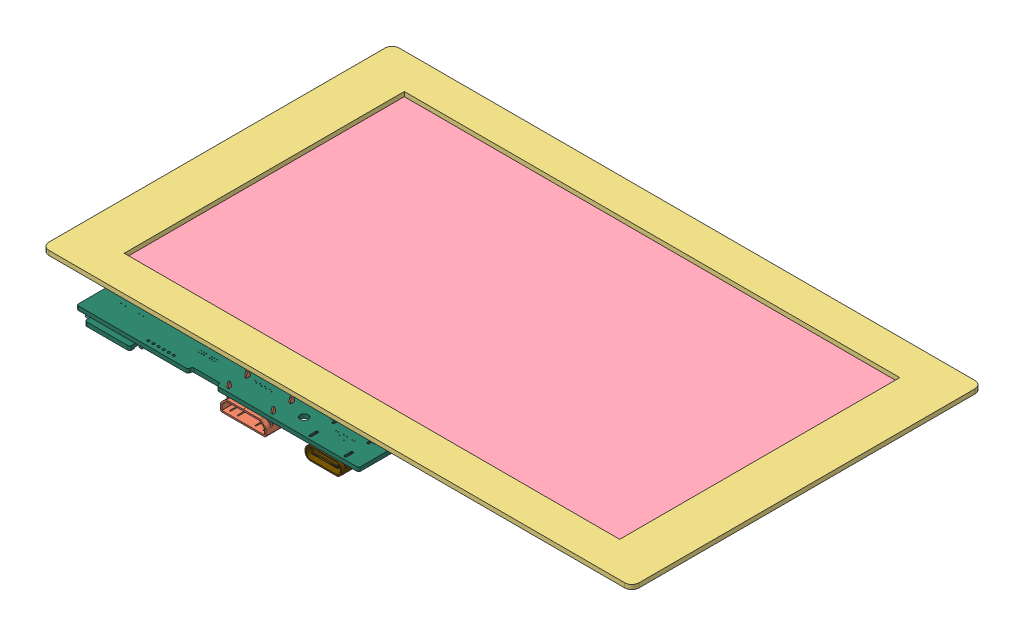
SolidWorks assembly Assembly Center Components, configuration Default. Lengths in mm. (continued)
Components (placement in the parent): (continued)
- Radxa CM3-1: Radxa CM3 [Default] at (-34.1679 -8.7691 -17.6603) x (0 0 -1) z (0 -1 0) size (40.05 55.02 3.7) (continued)
  - EMP_Models-1: EMP_Models [Default] at origin size (39.5 54.73 3.7) (continued)
    - C10-202: C10 [Default] at (-4.7475 1.3019 -1.2) x (-0.707107 -0.707107 0) z (0 0 -1) size (1.1 0.6 0.35)
    - C10-203: C10 [Default] at (0.9 2.95 -1.2) x (0.707107 -0.707107 0) z (0 0 -1) size (1.1 0.6 0.35)
    - C10-204: C10 [Default] at (4.05 11.1 -1.2) x (0 -1 0) z (0 0 -1) size (1.1 0.6 0.35)
    - D1-1: D1 [Default] at (13.3703 9.2021 0) x (-1 0 0) z (0 0 1) size (3.3 1.4 0.8)
    - D1-2: D1 [Default] at (15.4253 4.4887 0) x (0 -1 0) z (0 0 1) size (3.3 1.4 0.8)
    - ED8144-1: ED8144 [Default] at (-15.7 3.95 0) x (0 1 0) z (0 0 1) size (1.77 0.93 0.8)
    - ED8144-2: ED8144 [Default] at (-14.65 -20.2 0) size (1.77 0.93 0.8)
    - ED8144-3: ED8144 [Default] at (-2.4887 24.0177 0) x (0 1 0) z (0 0 1) size (1.77 0.93 0.8)
    - ED8147-1: ED8147 [Default] at (18.2193 9.1971 0) size (2.41 1.24 0.8)
    - ED8144-4: ED8144 [Default] at (17.6586 1.0982 0) x (0 -1 0) z (0 0 1) size (1.77 0.93 0.8)
    - ED8144-5: ED8144 [Default] at (17.6586 2.8762 0) x (0 1 0) z (0 0 1) size (1.77 0.93 0.8)
    - FB1-1: FB1 [Default] at (1.65 9.65 -1.2) x (1 0 0) z (0 0 -1) size (1.7 0.8 0.5)
    - FB1-2: FB1 [Default] at (9.4715 23.3369 0) x (0 1 0) z (0 0 1) size (1.7 0.8 0.5)
    - FB1-3: FB1 [Default] at (10.7443 20.4739 -1.2) x (1 0 0) z (0 0 -1) size (1.7 0.8 0.5)
    - FB1-4: FB1 [Default] at (9.7417 13.5389 -1.2) x (1 0 0) z (0 0 -1) size (1.7 0.8 0.5)
    - FB1-5: FB1 [Default] at (12.05 13.95 -1.2) x (0 -1 0) z (0 0 -1) size (1.7 0.8 0.5)
    - FB1-6: FB1 [Default] at (3.5025 2.1519 -1.2) x (-0.707107 0.707107 0) z (0 0 -1) size (1.7 0.8 0.5)
    - FB5-1: FB5 [Default] at (17.7525 -10.7981 0) x (0 -1 0) z (0 0 1) size (2.08 1.34 0.7)
    - FB5-2: FB5 [Default] at (16.3025 -10.7981 0) x (0 -1 0) z (0 0 1) size (2.08 1.34 0.7)
    - FB5-3: FB5 [Default] at (14.8525 -10.7981 0) x (0 -1 0) z (0 0 1) size (2.08 1.34 0.7)
    - FB5-4: FB5 [Default] at (13.4025 -10.7981 0) x (0 -1 0) z (0 0 1) size (2.08 1.34 0.7)
    - FB9-1: FB9 [Default] at (11.1972 22.9552 0) size (2.8 1.3 0.6)
    - J1-1: J1 [Default] at (11.3212 22.5507 -1.2) x (0 1 0) z (0 0 -1) size (2.84 22.55 1)
    - J90033-1: J90033 [Default] at (-13.7 5.05 0) x (0 1 0) z (0 0 1) size (4.08 2.13 0.5)
    - J90033-2: J90033 [Default] at (-16.8 -18.5 0) x (-1 0 0) z (0 0 1) size (4.08 2.13 0.5)
    - L1-1: L1 [Default] at (9.3525 -25.5481 0) x (0 1 0) z (0 0 1) size (2.78 2.28 1)
    - L10-1: L10 [Default] at (5.8 11.7 0) x (0 1 0) z (0 0 1) size (2.78 2.28 1)
    - L10-2: L10 [Default] at (12.0115 18.7649 0) size (2.78 2.28 1)
    - L10-3: L10 [Default] at (-0.9 20.75 0) x (0 1 0) z (0 0 1) size (2.78 2.28 1)
    - L13-1: L13 [Default] at (-13.7665 -4.2312 0) x (-0.707107 -0.707107 0) z (0 0 1) size (2.83 2.1 1.2)
    - L2-1: L2 [Default] at (-11.1177 21.5067 0) x (-0.707107 -0.707107 0) z (0 0 1) size (1.1 0.6 0.35)
    - L2-2: L2 [Default] at (-11.7527 23.4117 0) x (-1 0 0) z (0 0 1) size (1.1 0.6 0.35)
    - L10-4: L10 [Default] at (-17.3475 4.7519 0) x (0 -1 0) z (0 0 1) size (2.78 2.28 1)
    - L10-5: L10 [Default] at (18.3025 -19.6481 0) x (-1 0 0) z (0 0 1) size (2.78 2.28 1)
    - L10-6: L10 [Default] at (9.2 12.15 0) x (-1 0 0) z (0 0 1) size (2.78 2.28 1)
    - L10-7: L10 [Default] at (-0.85 16.7 0) x (0 1 0) z (0 0 1) size (2.78 2.28 1)
    - LED1-1: LED1 [Default] at (-2.8224 26.4941 0) x (-1 0 0) z (0 0 1) size (2.95 1.43 0.6)
    - M1-1: M1 [Default] at (-12.0975 -25.5981 -1.2) x (-1 0 0) z (0 0 -1) size (3.45 3.45 0.1)
    - M1-2: M1 [Default] at (12.2025 25.6519 0) size (3.45 3.45 0.1)
    - M1-3: M1 [Default] at (-12.0975 -25.5981 0) size (3.45 3.45 0.1)
    - M1-4: M1 [Default] at (12.2025 25.6519 -1.2) x (-1 0 0) z (0 0 -1) size (3.45 3.45 0.1)
    - Q4-1: Q4 [Default] at (-8.45 5.5 -1.2) x (-1 0 0) z (0 0 -1) size (1.27 1.32 0.8)
    - Q5-1: Q5 [Default] at (-7.3 23.05 0) size (3.35 3.3 1)
    - Q5-2: Q5 [Default] at (17 -3.9 0) x (-1 0 0) z (0 0 1) size (3.35 3.3 1)
    - R1-1: R1 [Default] at (6.8025 -4.5481 -1.2) x (1 0 0) z (0 0 -1) size (1.7 0.9 0.5)
    - L2-3: L2 [Default] at (12.9303 4.6718 -1.2) x (0 -1 0) z (0 0 -1) size (1.1 0.6 0.35)
    - L2-4: L2 [Default] at (17.75 -11.3 -1.2) x (0 1 0) z (0 0 -1) size (1.1 0.6 0.35)
    - L2-5: L2 [Default] at (17.75 -12.45 -1.2) x (0 1 0) z (0 0 -1) size (1.1 0.6 0.35)
    - L2-6: L2 [Default] at (15.7025 -17.9981 -1.2) x (0 1 0) z (0 0 -1) size (1.1 0.6 0.35)
    - L2-7: L2 [Default] at (18.45 -11.3 -1.2) x (0 1 0) z (0 0 -1) size (1.1 0.6 0.35)
    - L2-8: L2 [Default] at (18.45 -12.45 -1.2) x (0 1 0) z (0 0 -1) size (1.1 0.6 0.35)
    - L2-9: L2 [Default] at (15.0525 -17.9981 -1.2) x (0 1 0) z (0 0 -1) size (1.1 0.6 0.35)
    - L2-10: L2 [Default] at (15.0525 -19.1481 -1.2) x (0 1 0) z (0 0 -1) size (1.1 0.6 0.35)
    - L2-11: L2 [Default] at (13.7525 -17.9981 -1.2) x (0 1 0) z (0 0 -1) size (1.1 0.6 0.35)
    - L2-12: L2 [Default] at (13.7525 -19.1481 -1.2) x (0 1 0) z (0 0 -1) size (1.1 0.6 0.35)
    - R1-2: R1 [Default] at (12.7025 -9.6481 0) size (1.7 0.9 0.5)
    - L2-13: L2 [Default] at (0.4486 12.9437 -1.2) x (0 1 0) z (0 0 -1) size (1.1 0.6 0.35)
    - R1-3: R1 [Default] at (13.1025 -8.2481 0) x (0 -1 0) z (0 0 1) size (1.7 0.9 0.5)
    - L2-14: L2 [Default] at (14.4025 -17.9981 -1.2) x (0 1 0) z (0 0 -1) size (1.1 0.6 0.35)
    - L2-15: L2 [Default] at (14.4025 -19.1481 -1.2) x (0 1 0) z (0 0 -1) size (1.1 0.6 0.35)
    - R1-4: R1 [Default] at (12.9525 -11.8481 -1.2) x (-1 0 0) z (0 0 -1) size (1.7 0.9 0.5)
    - R1-5: R1 [Default] at (18.8525 -19.1481 -1.2) x (-1 0 0) z (0 0 -1) size (1.7 0.9 0.5)
    - L2-16: L2 [Default] at (11.8525 -13.8481 -1.2) x (0 -1 0) z (0 0 -1) size (1.1 0.6 0.35)
    - L2-17: L2 [Default] at (11.6025 -15.0981 -1.2) x (1 0 0) z (0 0 -1) size (1.1 0.6 0.35)
    - L2-18: L2 [Default] at (11.2025 -13.8481 -1.2) x (0 -1 0) z (0 0 -1) size (1.1 0.6 0.35)
    - L2-19: L2 [Default] at (11.7525 -16.2481 -1.2) x (-1 0 0) z (0 0 -1) size (1.1 0.6 0.35)
    - L2-20: L2 [Default] at (13.9025 -20.1981 0) x (0 -1 0) z (0 0 1) size (1.1 0.6 0.35)
    - R1-6: R1 [Default] at (11.8808 6.1274 0) size (1.7 0.9 0.5)
    - R1-7: R1 [Default] at (10.5014 7.0239 0) x (0 1 0) z (0 0 1) size (1.7 0.9 0.5)
    - L2-21: L2 [Default] at (-10.0048 -2.9217 0) x (-1 0 0) z (0 0 1) size (1.1 0.6 0.35)
    - L2-22: L2 [Default] at (-11.25 4.25 0) x (-0.707107 0.707107 0) z (0 0 1) size (1.1 0.6 0.35)
    - L2-23: L2 [Default] at (-7.55 2.1989 -1.2) x (1 0 0) z (0 0 -1) size (1.1 0.6 0.35)
    - L2-24: L2 [Default] at (18.2 -17.4 -1.2) x (-1 0 0) z (0 0 -1) size (1.1 0.6 0.35)
    - L2-25: L2 [Default] at (18.2 -16.75 -1.2) x (-1 0 0) z (0 0 -1) size (1.1 0.6 0.35)
    - L2-26: L2 [Default] at (19.25 -17.15 -1.2) x (0 -1 0) z (0 0 -1) size (1.1 0.6 0.35)
    - L2-27: L2 [Default] at (-13.3547 0.5177 0) x (-0.707107 -0.707107 0) z (0 0 1) size (1.1 0.6 0.35)
    - L2-28: L2 [Default] at (-3.95 9.75 0) x (0.707107 0.707107 0) z (0 0 1) size (1.1 0.6 0.35)
    - L2-29: L2 [Default] at (-7.45 4.9 -1.2) x (0 1 0) z (0 0 -1) size (1.1 0.6 0.35)
    - L2-30: L2 [Default] at (-3.35 10.8 0) x (0 1 0) z (0 0 1) size (1.1 0.6 0.35)
    - L2-31: L2 [Default] at (-8.9 -1.05 -1.2) x (0 1 0) z (0 0 -1) size (1.1 0.6 0.35)
    - L2-32: L2 [Default] at (-9.7407 -0.3884 -1.2) x (-1 0 0) z (0 0 -1) size (1.1 0.6 0.35)
    - L2-33: L2 [Default] at (1.5025 -5.4481 -1.2) x (-0.707107 -0.707107 0) z (0 0 -1) size (1.1 0.6 0.35)
    - L2-34: L2 [Default] at (-9.7625 1.3757 -1.2) x (1 0 0) z (0 0 -1) size (1.1 0.6 0.35)
    - L2-35: L2 [Default] at (-9.7722 0.251 -1.2) x (1 0 0) z (0 0 -1) size (1.1 0.6 0.35)
    - L2-36: L2 [Default] at (8.8525 -3.8481 -1.2) x (1 0 0) z (0 0 -1) size (1.1 0.6 0.35)
    - L2-37: L2 [Default] at (8.8525 -4.4981 -1.2) x (1 0 0) z (0 0 -1) size (1.1 0.6 0.35)
    - R24-1: R24 [Default] at (13.5019 5.7507 0) x (0 -1 0) z (0 0 1) size (2.5 1.3 0.6)
    - L2-38: L2 [Default] at (8.8525 -5.1481 -1.2) x (1 0 0) z (0 0 -1) size (1.1 0.6 0.35)
    - R1-8: R1 [Default] at (11.8808 7.9054 0) x (-1 0 0) z (0 0 1) size (1.7 0.9 0.5)
    - L2-39: L2 [Default] at (8.839 -5.6572 -1.2) x (-1 0 0) z (0 0 -1) size (1.1 0.6 0.35)
    - L2-40: L2 [Default] at (13.5019 8.1637 0) size (1.1 0.6 0.35)
    - R1-9: R1 [Default] at (11.8808 7.0164 0) x (-1 0 0) z (0 0 1) size (1.7 0.9 0.5)
    - L2-41: L2 [Default] at (1.9025 -4.5981 -1.2) x (-0.707107 0.707107 0) z (0 0 -1) size (1.1 0.6 0.35)
    - R1-10: R1 [Default] at (12.4 10.2 -1.2) x (-1 0 0) z (0 0 -1) size (1.7 0.9 0.5)
    - R1-11: R1 [Default] at (12.4278 9.235 -1.2) x (-1 0 0) z (0 0 -1) size (1.7 0.9 0.5)
    - L2-42: L2 [Default] at (0.0025 12.7519 0) x (0.707107 0.707107 0) z (0 0 1) size (1.1 0.6 0.35)
    - L2-43: L2 [Default] at (0.4393 12.3013 0) x (0.707107 0.707107 0) z (0 0 1) size (1.1 0.6 0.35)
    - L2-44: L2 [Default] at (0.9525 11.8019 0) x (0.707107 0.707107 0) z (0 0 1) size (1.1 0.6 0.35)
    - L2-45: L2 [Default] at (1.3881 11.3747 0) x (0.707107 0.707107 0) z (0 0 1) size (1.1 0.6 0.35)
    - L2-46: L2 [Default] at (1.9025 10.8519 0) x (0.707107 0.707107 0) z (0 0 1) size (1.1 0.6 0.35)
    - L2-47: L2 [Default] at (2.3296 10.4351 0) x (0.707107 0.707107 0) z (0 0 1) size (1.1 0.6 0.35)
    - L2-48: L2 [Default] at (2.8525 9.9019 0) x (0.707107 0.707107 0) z (0 0 1) size (1.1 0.6 0.35)
    - L2-49: L2 [Default] at (3.2748 9.4731 0) x (0.707107 0.707107 0) z (0 0 1) size (1.1 0.6 0.35)
    - L2-50: L2 [Default] at (-4.75 10.35 0) x (-1 0 0) z (0 0 1) size (1.1 0.6 0.35)
    - L2-51: L2 [Default] at (1.1909 6.5961 -1.2) x (0 -1 0) z (0 0 -1) size (1.1 0.6 0.35)
    - L2-52: L2 [Default] at (10.3525 2.1019 0) x (-0.707107 0.707107 0) z (0 0 1) size (1.1 0.6 0.35)
    - R1-12: R1 [Default] at (9.9432 9.4653 0) size (1.7 0.9 0.5)
    - R1-13: R1 [Default] at (9.5622 8.0683 0) x (0 -1 0) z (0 0 1) size (1.7 0.9 0.5)
    - L2-53: L2 [Default] at (-8.7065 -3.7391 0) size (1.1 0.6 0.35)
    - L2-54: L2 [Default] at (-8.7065 -4.3741 0) size (1.1 0.6 0.35)
    - L2-55: L2 [Default] at (-6.5975 -2.9981 -1.2) x (-0.707107 -0.707107 0) z (0 0 -1) size (1.1 0.6 0.35)
    - R1-14: R1 [Default] at (-15.4372 0.8153 0) x (-1 0 0) z (0 0 1) size (1.7 0.9 0.5)
    - L2-56: L2 [Default] at (-18.76 -2.973 0) x (-0.707107 0.707107 0) z (0 0 1) size (1.1 0.6 0.35)
    - R1-15: R1 [Default] at (-15.0359 2.0509 0) x (0 1 0) z (0 0 1) size (1.7 0.9 0.5)
    - L2-57: L2 [Default] at (-5.15 9.75 0) x (-1 0 0) z (0 0 1) size (1.1 0.6 0.35)
    - L2-58: L2 [Default] at (-18.3381 -2.5736 0) x (0.707107 -0.707107 0) z (0 0 1) size (1.1 0.6 0.35)
    - L2-59: L2 [Default] at (5.8025 -20.8481 -1.2) x (1 0 0) z (0 0 -1) size (1.1 0.6 0.35)
    - L2-60: L2 [Default] at (5.8025 -20.1981 -1.2) x (1 0 0) z (0 0 -1) size (1.1 0.6 0.35)
    - R24-2: R24 [Default] at (11.9025 -23.7981 -1.2) x (-1 0 0) z (0 0 -1) size (2.5 1.3 0.6)
    - R1-16: R1 [Default] at (-13.55 -21.25 -1.2) x (1 0 0) z (0 0 -1) size (1.7 0.9 0.5)
    - R24-3: R24 [Default] at (7.0025 -26.5481 -1.2) x (-1 0 0) z (0 0 -1) size (2.5 1.3 0.6)
    - R1-17: R1 [Default] at (-13.55 -20.3 -1.2) x (1 0 0) z (0 0 -1) size (1.7 0.9 0.5)
    - L2-61: L2 [Default] at (11.5525 -21.7481 0) size (1.1 0.6 0.35)
    - L2-62: L2 [Default] at (12.7525 -26.2481 -1.2) x (1 0 0) z (0 0 -1) size (1.1 0.6 0.35)
    - L2-63: L2 [Default] at (-18.4 -16.6 -1.2) x (1 0 0) z (0 0 -1) size (1.1 0.6 0.35)
    - L2-64: L2 [Default] at (-1.6 13.75 0) x (0 1 0) z (0 0 1) size (1.1 0.6 0.35)
    - L2-65: L2 [Default] at (13.9525 -26.8981 0) size (1.1 0.6 0.35)
    - L2-66: L2 [Default] at (-12.014 6.1193 -1.2) x (0 1 0) z (0 0 -1) size (1.1 0.6 0.35)
    - L2-67: L2 [Default] at (-10.4 5.9 -1.2) x (0 1 0) z (0 0 -1) size (1.1 0.6 0.35)
    - L2-68: L2 [Default] at (-12.6417 6.1168 -1.2) x (0 1 0) z (0 0 -1) size (1.1 0.6 0.35)
    - L2-69: L2 [Default] at (-11.4087 6.1174 -1.2) x (0 1 0) z (0 0 -1) size (1.1 0.6 0.35)
    - L2-70: L2 [Default] at (-12.6469 -1.643 -1.2) x (1 0 0) z (0 0 -1) size (1.1 0.6 0.35)
    - L2-71: L2 [Default] at (13.1198 7.7736 -1.2) x (1 0 0) z (0 0 -1) size (1.1 0.6 0.35)
    - L2-72: L2 [Default] at (-16.9 -11.65 -1.2) x (-1 0 0) z (0 0 -1) size (1.1 0.6 0.35)
    - L2-73: L2 [Default] at (-18.1 -11.65 -1.2) x (1 0 0) z (0 0 -1) size (1.1 0.6 0.35)
    - L2-74: L2 [Default] at (-15.6 -15.95 -1.2) x (-1 0 0) z (0 0 -1) size (1.1 0.6 0.35)
    - L2-75: L2 [Default] at (-12.55 0.45 -1.2) x (-1 0 0) z (0 0 -1) size (1.1 0.6 0.35)
    - L2-76: L2 [Default] at (-13.55 0.45 -1.2) x (-1 0 0) z (0 0 -1) size (1.1 0.6 0.35)
    - R24-4: R24 [Default] at (-14.4732 17.1388 -1.2) x (0 1 0) z (0 0 -1) size (2.5 1.3 0.6)
    - L2-77: L2 [Default] at (-17.707 19.6733 -1.2) x (1 0 0) z (0 0 -1) size (1.1 0.6 0.35)
    - L2-78: L2 [Default] at (13.1107 8.3605 -1.2) x (1 0 0) z (0 0 -1) size (1.1 0.6 0.35)
    - L2-79: L2 [Default] at (-17.7116 19.1714 -1.2) x (-1 0 0) z (0 0 -1) size (1.1 0.6 0.35)
    - L2-80: L2 [Default] at (-12.999 2.1325 0) x (-1 0 0) z (0 0 1) size (1.1 0.6 0.35)
    - L2-81: L2 [Default] at (-5.9125 16.7079 0) x (0 1 0) z (0 0 1) size (1.1 0.6 0.35)
    - L2-82: L2 [Default] at (-18.8975 5.2019 0) x (0 -1 0) z (0 0 1) size (1.1 0.6 0.35)
    - R1-18: R1 [Default] at (-17.0263 0.7967 0) size (1.7 0.9 0.5)
    - R1-19: R1 [Default] at (-16.2916 2.0337 0) x (0 1 0) z (0 0 1) size (1.7 0.9 0.5)
    - L2-83: L2 [Default] at (-11.7975 6.8019 0) size (1.1 0.6 0.35)
    - L2-84: L2 [Default] at (18.85 -12.45 0) size (1.1 0.6 0.35)
    - L2-85: L2 [Default] at (18.85 -11.8 0) size (1.1 0.6 0.35)
    - L2-86: L2 [Default] at (12.2953 4.6718 -1.2) x (0 -1 0) z (0 0 -1) size (1.1 0.6 0.35)
    - L2-87: L2 [Default] at (18.85 -13.1 0) size (1.1 0.6 0.35)
    - L2-88: L2 [Default] at (18.1 -0.6 0) x (0 1 0) z (0 0 1) size (1.1 0.6 0.35)
    - L2-89: L2 [Default] at (17.45 -0.6 0) x (0 1 0) z (0 0 1) size (1.1 0.6 0.35)
    - L2-90: L2 [Default] at (18.2 -15.45 -1.2) x (1 0 0) z (0 0 -1) size (1.1 0.6 0.35)
    - L2-91: L2 [Default] at (9.0525 1.2019 -1.2) x (-1 0 0) z (0 0 -1) size (1.1 0.6 0.35)
    - L2-92: L2 [Default] at (-10.2001 3.3697 -1.2) x (0 1 0) z (0 0 -1) size (1.1 0.6 0.35)
    - L2-93: L2 [Default] at (-16.15 -20.2 0) size (1.1 0.6 0.35)
    - R24-5: R24 [Default] at (-8.1 25.45 0) x (-1 0 0) z (0 0 1) size (2.5 1.3 0.6)
    - L2-94: L2 [Default] at (11.7 13.4 0) x (0 1 0) z (0 0 1) size (1.1 0.6 0.35)
    - L2-95: L2 [Default] at (3.95 11.85 0) x (-1 0 0) z (0 0 1) size (1.1 0.6 0.35)
    - L2-96: L2 [Default] at (10.8685 18.0306 -1.2) x (-1 0 0) z (0 0 -1) size (1.1 0.6 0.35)
    - L2-97: L2 [Default] at (8.5825 18.5109 -1.2) x (-1 0 0) z (0 0 -1) size (1.1 0.6 0.35)
    - L2-98: L2 [Default] at (5.9323 23.8177 0) x (0 -1 0) z (0 0 1) size (1.1 0.6 0.35)
    - L2-99: L2 [Default] at (5.2823 23.8177 0) x (0 -1 0) z (0 0 1) size (1.1 0.6 0.35)
    - L2-100: L2 [Default] at (-8.8 24.55 0) x (-1 0 0) z (0 0 1) size (1.1 0.6 0.35)
    - R9216-1: R9216 [Default] at (3.3 18.2 -1.2) x (1 0 0) z (0 0 -1) size (3.6 2.1 0.8)
    - L2-101: L2 [Default] at (-0.3818 13.9135 -1.2) x (0 1 0) z (0 0 -1) size (1.1 0.6 0.35)
    - L2-102: L2 [Default] at (0.45 16.7 -1.2) x (-1 0 0) z (0 0 -1) size (1.1 0.6 0.35)
    - L2-103: L2 [Default] at (-0.3818 14.9291 -1.2) x (0 1 0) z (0 0 -1) size (1.1 0.6 0.35)
    - L2-104: L2 [Default] at (0.55 14.45 -1.2) x (-1 0 0) z (0 0 -1) size (1.1 0.6 0.35)
    - L2-105: L2 [Default] at (-1.1 14.15 0) x (0 -1 0) z (0 0 1) size (1.1 0.6 0.35)
    - L2-106: L2 [Default] at (0.75 14.6 0) x (0 1 0) z (0 0 1) size (1.1 0.6 0.35)
    - L2-107: L2 [Default] at (-3.9887 23.8177 0) x (0 1 0) z (0 0 1) size (1.1 0.6 0.35)
    - R9216-2: R9216 [Default] at (16.5683 7.4937 0) x (-1 0 0) z (0 0 1) size (3.6 2.1 0.8)
    - L2-108: L2 [Default] at (-18.0618 -3.6891 0) x (0.707107 -0.707107 0) z (0 0 1) size (1.1 0.6 0.35)
    - L2-109: L2 [Default] at (-16.8694 -1.2155 0) x (-0.707107 -0.707107 0) z (0 0 1) size (1.1 0.6 0.35)
    - L2-110: L2 [Default] at (-18.4855 -4.1201 0) x (0.707107 -0.707107 0) z (0 0 1) size (1.1 0.6 0.35)
    - R1-20: R1 [Default] at (4.2 12.6 -1.2) x (0 1 0) z (0 0 -1) size (1.7 0.9 0.5)
    - R1-21: R1 [Default] at (2.6 12.6 -1.2) x (0 1 0) z (0 0 -1) size (1.7 0.9 0.5)
    - R1-22: R1 [Default] at (5 12.6 -1.2) x (0 1 0) z (0 0 -1) size (1.7 0.9 0.5)
    - R1-23: R1 [Default] at (9.8 14.3 -1.2) x (-1 0 0) z (0 0 -1) size (1.7 0.9 0.5)
    - R1-24: R1 [Default] at (-18.35 1.2 0) x (0 1 0) z (0 0 1) size (1.7 0.9 0.5)
    - R1-25: R1 [Default] at (3.4 12.6 -1.2) x (0 1 0) z (0 0 -1) size (1.7 0.9 0.5)
    - L2-111: L2 [Default] at (-3.1812 25.4157 0) size (1.1 0.6 0.35)
    - L2-112: L2 [Default] at (15.7205 1.3062 0) size (1.1 0.6 0.35)
    - L2-113: L2 [Default] at (15.7205 1.9412 0) size (1.1 0.6 0.35)
    - L2-114: L2 [Default] at (14.7219 1.3075 0) x (-1 0 0) z (0 0 1) size (1.1 0.6 0.35)
    - L2-115: L2 [Default] at (14.9 -3.05 0) x (0 -1 0) z (0 0 1) size (1.1 0.6 0.35)
    - L2-116: L2 [Default] at (17.7 -1.55 0) size (1.1 0.6 0.35)
    - L2-117: L2 [Default] at (-7.95 26.5 0) x (-1 0 0) z (0 0 1) size (1.1 0.6 0.35)
    - L2-118: L2 [Default] at (-9 1.15 -1.2) x (0 1 0) z (0 0 -1) size (1.1 0.6 0.35)
    - L2-119: L2 [Default] at (17.5 -14.2 -1.2) x (-1 0 0) z (0 0 -1) size (1.1 0.6 0.35)
    - L2-120: L2 [Default] at (13.1025 -19.1481 -1.2) x (0 1 0) z (0 0 -1) size (1.1 0.6 0.35)
    - L2-121: L2 [Default] at (19.15 -11.3 -1.2) x (0 1 0) z (0 0 -1) size (1.1 0.6 0.35)
    - L2-122: L2 [Default] at (19.15 -12.45 -1.2) x (0 1 0) z (0 0 -1) size (1.1 0.6 0.35)
    - L2-123: L2 [Default] at (18.7525 -17.9981 0) size (1.1 0.6 0.35)
    - L2-124: L2 [Default] at (15.2025 -20.1981 0) x (0 -1 0) z (0 0 1) size (1.1 0.6 0.35)
    - L2-125: L2 [Default] at (14.0025 -20.0481 -1.2) x (1 0 0) z (0 0 -1) size (1.1 0.6 0.35)
    - TP1-1: TP1 [Default] at (-12.0342 7.0446 -1.2) x (-1 0 0) z (0 0 -1) size (1 1 0.1)
    - TP1-2: TP1 [Default] at (18.7 0.35 0) size (1 1 0.1)
    - TP1-3: TP1 [Default] at (-7 3 -1.2) x (-0.707107 0.707107 0) z (0 0 -1) size (1 1 0.1)
    - TP1-4: TP1 [Default] at (18.75 13.45 -1.2) x (-1 0 0) z (0 0 -1) size (1 1 0.1)
    - TP1-5: TP1 [Default] at (19.4 9.05 -1.2) x (-1 0 0) z (0 0 -1) size (1 1 0.1)
    - TP1-6: TP1 [Default] at (19.4 10.6 -1.2) x (-1 0 0) z (0 0 -1) size (1 1 0.1)
    - TP1-7: TP1 [Default] at (-18.6 -15.75 -1.2) x (-1 0 0) z (0 0 -1) size (1 1 0.1)
    - TP1-8: TP1 [Default] at (-17.5 -15.75 -1.2) x (-1 0 0) z (0 0 -1) size (1 1 0.1)
    - TP1-9: TP1 [Default] at (14.35 -10.85 -1.2) x (-1 0 0) z (0 0 -1) size (1 1 0.1)
    - TP1-10: TP1 [Default] at (-8.8451 3.2927 -1.2) x (-1 0 0) z (0 0 -1) size (1 1 0.1)
    - TP1-11: TP1 [Default] at (4.5413 20.3907 -1.2) x (-1 0 0) z (0 0 -1) size (1 1 0.1)
    - TP1-12: TP1 [Default] at (18.6825 1.3989 0) size (1 1 0.1)
    - TP1-13: TP1 [Default] at (18.6825 2.4489 0) size (1 1 0.1)
    - U1-1: U1 [Default] at (-0.1975 0.4519 0) x (-0.707107 0.707107 0) z (0 0 1) size (18.71 17.21 1.1)
    - U2-1: U2 [Default] at (-1.0248 -19.8218 0) x (0 -1 0) z (0 0 1) size (13.49 18.53 1)
    - U3-1: U3 [Default] at (12.9025 -23.7481 0) x (0 -1 0) z (0 0 1) size (4.03 3.13 1)
    - U3-2: U3 [Default] at (-18.15 -19.4 -1.2) x (1 0 0) z (0 0 -1) size (4.03 3.13 1)
    - U4300-1: U4300 [Default] at (-16.9 -13.45 0) x (-1 0 0) z (0 0 1) size (5.99 7 1.2)
    - U4301-1: U4301 [Default] at (5.2805 18.1299 0) x (0 1 0) z (0 0 1) size (8.35 8.35 0.8)
    - U4302-1: U4302 [Default] at (-16.4535 -5.0091 0) x (0.707107 0.707107 0) z (0 0 1) size (1.93 2.38 0.8)
    - U5-1: U5 [Default] at (-7.6975 14.2519 -1.2) x (1 0 0) z (0 0 -1) size (11.63 13.5 1.2)
    - U7-1: U7 [Default] at (14.2608 3.741 0) x (0 -1 0) z (0 0 1) size (2.08 2.45 0.7)
    - U8-1: U8 [Default] at (-12.9975 13.9519 0) x (0 -1 0) z (0 0 1) size (13.66 12.7 1.3)
    - U9-1: U9 [Default] at (15.3025 -15.6981 0) x (0 -1 0) z (0 0 1) size (5.84 5.5 1)
    - U3-3: U3 [Default] at (13.5 0.3 0) size (4.03 3.13 1)
    - Y1-1: Y1 [Default] at (-4.2838 13.1005 0) x (-1 0 0) z (0 0 1) size (3.6 3.57 1.2)
    - Y1-2: Y1 [Default] at (-17.6116 16.6641 -1.2) x (-1 0 0) z (0 0 -1) size (3.6 3.57 1.2)
    - Y1-3: Y1 [Default] at (17.8 -7.6 0) x (0 -1 0) z (0 0 1) size (3.6 3.57 1.2)
    - Y4-1: Y4 [Default] at (-0.81 24.6548 0) size (3.6 1.7 1.2)
  - Board_outline(1)-1: Board_outline(1) [Default] at origin size (40.05 55.02 1.2)
- User Library-CR1225 v1-1: User Library-CR1225 v1 [Default] at (-65.8849 -7.0512 19.9145) x (0 0 -1) z (0 -1 0) size (12.4 12.4 2.5)
  - refine_Revolution001-1: refine_Revolution001 [Default] at (0 0 2.5) x (1 0 0) z (0 1 0) size (10.2 0.85 10.2)
  - refine_Cut001-1: refine_Cut001 [Default] at (0 1 2.5) x (1 0 0) z (0 1 0) size (12.4 2.5 12.4)
- 5040500491 v1-1: 5040500491 v1 [Default] at (-31.1609 -7.15 36.6709) x (-1 0 0) z (0 -1 0) size (10.55 6.44 2)
  - 5040500491-1: 5040500491 [Default] at origin size (10.55 6.44 2)
- DF40C-100DS-1: DF40C-100DS [Default] at (-37.655 -6.2 -0.495) x (0 0 -1) z (-1 0 0) size (3.49 2 22.61)
- DF40C-100DS-2: DF40C-100DS [Default] at (-37.655 -6.2 -34.495) x (0 0 -1) z (-1 0 0) size (3.49 2 22.61)
- Micro SD-Card-1: Micro SD-Card [Default] at (-52.45 -7.1 39.52) x (0 0 -1) z (-1 0 0) size (15 1.01 11)
- CUI_DEVICES_SJ-43516-SMT-TR-1: CUI_DEVICES_SJ-43516-SMT-TR [Default] at (-2.55 -8.65 -45.17) x (0 0 -1) z (-1 0 0) size (19.2 5.8 9)
- PCIe Slot  v1-1: PCIe Slot  v1 [Default] at (-9.09 -6.1502 6.7) x (-1 0 0) z (0 0 1) size (22 4.8 8.55)
- 1054500101 v1-1: 1054500101 v1 [Default] at (0 -7.7798 41.669) x (1 0 0) z (0 -1 0) size (8.94 7.9 3.96)
- 502570-0893 v1-1: 502570-0893 v1 [Default] at (-97.1844 -7.0502 -24.8743) x (1 0 0) z (0 -1 0) size (13.8 15.5 1.8)
- 9774025243R (rev1) v1-1: 9774025243R (rev1) v1 [Default] at (0 -52.8238 2.1762) x (1 0 0) z (0 -1 0) size (4.35 4.35 3.9)
- DF40C-100DS-3: DF40C-100DS [Default] at (-9.8603 -6.2 -23.511) x (1 0 0) z (0 0 -1) size (3.49 2 22.61)
- 5051100892 v1-1: 5051100892 v1 [Default] at (-65.4404 -6.1942 -19.6945) x (0 0 1) z (1 0 0) size (9.5 1.9 5.3)
- keystone-PN1072TR v1-1: keystone-PN1072TR v1 [Default] at (-72.6801 -0.2846 31.6836) x (1 0 0) z (0 0 -1) size (10.39 4.4 15.9)
- TPS65987DDHRSHR--3DModel-STEP-56544 v1-1: TPS65987DDHRSHR--3DModel-STEP-56544 v1 [Default] at (-12.5607 -6.1 22.9561) x (-1 0 0) z (0 0 1) size (7 1 7)
- TPD4E05U06DQAR--3DModel-STEP-56544 v1-1: TPD4E05U06DQAR--3DModel-STEP-56544 v1 [Default] at (4.7671 -6.1 32.9073) x (0 0 1) z (1 0 0) size (1 0.55 2.5)
- TPD4E05U06DQAR--3DModel-STEP-56544 v1-2: TPD4E05U06DQAR--3DModel-STEP-56544 v1 [Default] at (-3.01 -6.1 32.9073) x (0 0 1) z (1 0 0) size (1 0.55 2.5)
- TSIC 306 SOP-8--3DModel-STEP-510211 v1-1: TSIC 306 SOP-8--3DModel-STEP-510211 v1 [Default] at (-60.1923 -6.1499 6.8931) x (-1 0 0) z (0 0 1) size (5.99 1.73 4.93)
- 5034801700 v1-1: 5034801700 v1 [Default] at (6.9127 -6.1711 10.2732) x (0 0 1) z (1 0 0) size (10.2 1.87 3.6)
- 5034801700 v1-2: 5034801700 v1 [Default] at (-25.1264 -6.1711 10.2943) x (0 0 -1) z (-1 0 0) size (10.2 1.87 3.6)
- VLCF4020T-220MR56--3DModel-STEP-56544 v1-1: VLCF4020T-220MR56--3DModel-STEP-56544 v1 [Default] at (-60.5998 -6.1052 -39.9462) x (0 0 -1) z (-1 0 0) size (4 2.02 4.05)
- Heatsink-V2 v1-1: Heatsink-V2 v1 [Default] at (-21.2372 -13.3527 3.8484) x (0 0 -1) z (1 0 0) size (46.85 6 53)
- QFN_GEFLRV_CIR v1-1: QFN_GEFLRV_CIR v1 [Default] at (0.5729 -5.758 -18.9632) x (1 0 0) z (0 -1 0) size (5 5 0.99)
- 505110-3091 v1-1: 505110-3091 v1 [Default] at (-70.5178 -6.0871 -0.2937) x (0 0 1) z (1 0 0) size (20.5 1.9 5.3)
- ASPI-0630HI v1-1: ASPI-0630HI v1 [Default] at (-31.1721 -7.6525 20.8058) x (-1 0 0) z (0 0 1) size (7.2 3 6.65)
- Retro Lite CM5 (Latest)-18-1: Retro Lite CM5 (Latest)-18 [Default] at origin size (60.98 9.58 0.4)
- Retro Lite CM5 Carrier Board_CM5IO_Mapping_X2.0 v3-1: Retro Lite CM5 Carrier Board_CM5IO_Mapping_X2.0 v3 [Default] at (-1.05 -5.1782 42.5) x (-1 0 0) z (0 -1 0) size (82.67 91.25 0.97)
  - Retro Lite CM5 Carrier Board_CM5IO_Mapping_X2.0 v3(2)^Retro Lite CM5 Carrier Board_CM5IO_Mapping_X2.0 v3-1: Retro Lite CM5 Carrier Board_CM5IO_Mapping_X2.0 v3(2)^Retro Lite CM5 Carrier Board_CM5IO_Mapping_X2.0 v3 [Default] at origin size (82.67 91.25 0.97) (virtual)
    - Board^Retro Lite CM5 Carrier Board_CM5IO_Mapping_X2.0 v3(2)_Retro Lite CM5 Carrier Board_CM5IO_Mapping_X2.0 v3-1: Board^Retro Lite CM5 Carrier Board_CM5IO_Mapping_X2.0 v3(2)_Retro Lite CM5 Carrier Board_CM5IO_Mapping_X2.0 v3 [Default] at origin size (82.67 91.25 0.97) (virtual)
Mates (geometry in assembly coordinates):
- Concentric1: concentric aligned: cylinder of Retro Lite CM5 Carrier Board_CM5IO_Mapping_X2.0 v2 (1)-1/Board (36)-1 through (-72.8 -5.1782 18.5) axis (0 -1 0) radius 1; cylinder of Retro Lite CM5 Carrier Board_CM5IO_Mapping_X2.0 v3-1/Retro Lite CM5 Carrier Board_CM5IO_Mapping_X2.0 v3(2)^Retro Lite CM5 Carrier Board_CM5IO_Mapping_X2.0 v3-1/Board^Retro Lite CM5 Carrier Board_CM5IO_Mapping_X2.0 v3(2)_Retro Lite CM5 Carrier Board_CM5IO_Mapping_X2.0 v3-1 through (-72.8 -5.1782 18.5) axis (0 -1 0) radius 1
- Concentric2: concentric aligned: cylinder of Retro Lite CM5 Carrier Board_CM5IO_Mapping_X2.0 v2 (1)-1/Board (36)-1 through (-9.09 -5.1782 -40.5) axis (0 -1 0) radius 1; cylinder of Retro Lite CM5 Carrier Board_CM5IO_Mapping_X2.0 v3-1/Retro Lite CM5 Carrier Board_CM5IO_Mapping_X2.0 v3(2)^Retro Lite CM5 Carrier Board_CM5IO_Mapping_X2.0 v3-1/Board^Retro Lite CM5 Carrier Board_CM5IO_Mapping_X2.0 v3(2)_Retro Lite CM5 Carrier Board_CM5IO_Mapping_X2.0 v3-1 through (-9.09 -5.1782 -40.5) axis (0 -1 0) radius 1
- Coincident1: coincident aligned: plane of Retro Lite CM5 Carrier Board_CM5IO_Mapping_X2.0 v2 (1)-1/Board (36)-1 through (-32.9322 -6.1502 0.4989) normal (0 -1 0); plane of Retro Lite CM5 Carrier Board_CM5IO_Mapping_X2.0 v3-1/Retro Lite CM5 Carrier Board_CM5IO_Mapping_X2.0 v3(2)^Retro Lite CM5 Carrier Board_CM5IO_Mapping_X2.0 v3-1/Board^Retro Lite CM5 Carrier Board_CM5IO_Mapping_X2.0 v3(2)_Retro Lite CM5 Carrier Board_CM5IO_Mapping_X2.0 v3-1 through (-32.9322 -6.1502 0.4539) normal (0 -1 0)
